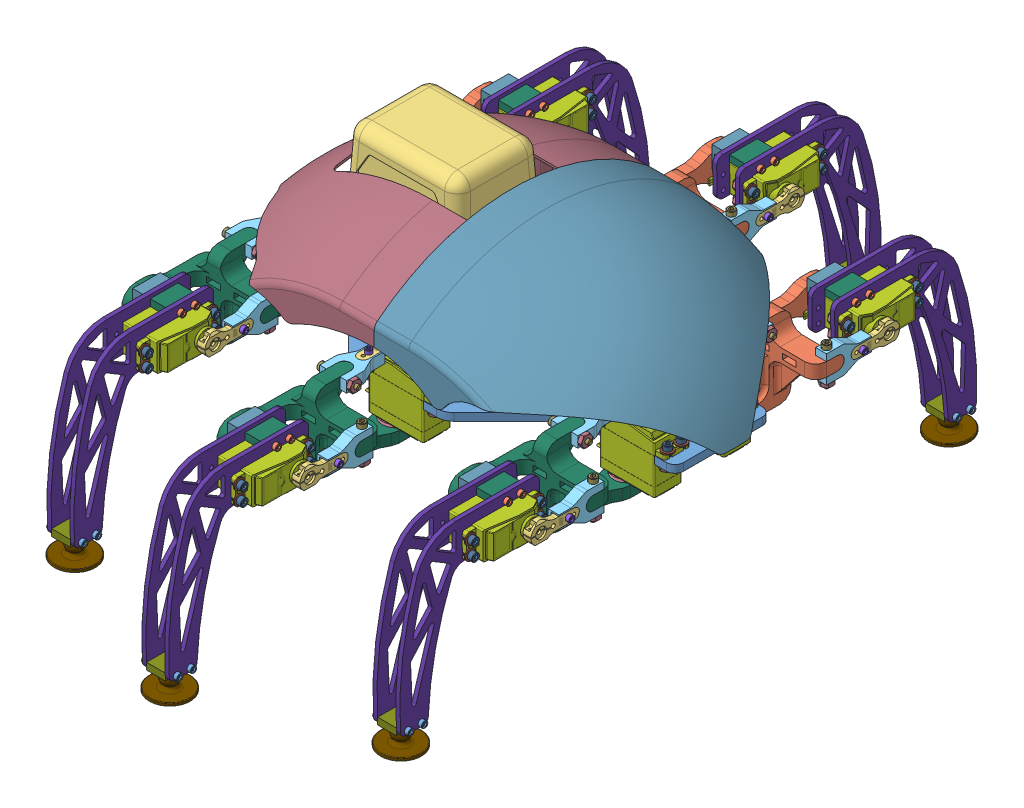
SolidWorks assembly Hexapod_(Small), configuration Défaut. Lengths in mm. (continued)
Mates (geometry in assembly coordinates):
- Coincident2: coincident anti-aligned: plane of Body_(Small)-5 through (-295 -5.601 0) normal (0 0 -1)
- Coincident3: coincident aligned: plane of Body_(Small)-5 through (-310 0 15.2) normal (0 1 0)
- Coincident4: coincident aligned: plane of Body_(Small)-5 through (0 0 50.6) normal (1 0 0)
- Coïncidente2: coincident anti-aligned: plane of arduinoMega-1 through (-199.11 -5.6 14.42) normal (0 1 0); plane of Body_(Small)-5 through (-310 -5.6 15.2) normal (0 -1 0)
- Coïncidente4: coincident anti-aligned: plane of Body_(Small)-5 through (-310 -5.6 15.2) normal (0 -1 0); plane of 12Channel PWM-1 through (-154.8 -5.6 -12.75) normal (0 1 0)
- Coïncidente5: coincident anti-aligned: plane of Body_(Small)-5 through (-310 -5.6 15.2) normal (0 -1 0); plane of DROK_090483.stp-1 through (-99 -5.6 15.2) normal (0 1 0)
- Parallèle4: parallel aligned: plane of Body_(Small)-5 through (0 0 50.6) normal (1 0 0); plane of 12Channel PWM-1 through (-132.7 -7.1 -12.75) normal (1 0 0)
- Concentric13: concentric aligned: cylinder of Body_(Small)-5 through (-154.8 0 43.15) axis (0 -1 0) radius 1.25; cylinder of 12Channel PWM-1 through (-154.8 -2.0645 43.15) axis (0 -1 0) radius 1.25
- Concentric17: concentric anti-aligned: circle of Body-1; circle of DROK_090483.stp-1
- Concentric18: concentric aligned: cylinder of Body_(Small)-5 through (-80.685 0 41.615) axis (0 -1 0) radius 1.45; cylinder of DROK_090483.stp-1 through (-80.685 -5.6 41.615) axis (0 -1 0) radius 1.585
- Concentric19: concentric aligned: cylinder of Body_(Small)-5 through (-175 0 -26.2) axis (0 -1 0) radius 1.6; circle of arduinoMega-1
- Concentric22: concentric aligned: cylinder of Body_(Small)-5 through (-223.22 0 49.91) axis (0 -1 0) radius 1.6; cylinder of arduinoMega-1 through (-223.22 -7.6 49.91) axis (0 -1 0) radius 1.6
- Concentric23: concentric anti-aligned: cylinder of Body_(Small)-5 through (-40.288 0 19.69) axis (0 -1 0) radius 1.45; cylinder of HX-SHCS 0.138-32x0.625x0.625-N-2 through (-40.288 35.2552 19.69) axis (0 1 0) radius 1.7526
- Concentric24: concentric anti-aligned: cylinder of Body_(Small)-5 through (-50.288 0 19.69) axis (0 -1 0) radius 1.45; cylinder of HX-SHCS 0.138-32x0.625x0.625-N-3 through (-50.288 35.2552 19.69) axis (0 1 0) radius 1.7526
- Coincident19: coincident anti-aligned: plane of Body_(Small)-5 through (-310 0 15.2) normal (0 1 0); plane of HX-SHCS 0.138-32x0.625x0.625-N-2 through (-40.288 0 16.8198) normal (0 -1 0)
- Coincident20: coincident anti-aligned: plane of Body_(Small)-5 through (-310 0 15.2) normal (0 1 0); plane of HX-SHCS 0.138-32x0.625x0.625-N-3 through (-47.8023 0 18.2549) normal (0 -1 0)
- Parallel10: parallel aligned: plane of Body_(Small)-5 through (0 0 50.6) normal (1 0 0); plane of HX-SHCS 0.138-32x0.625x0.625-N-3 through (-51.6723 1.8796 20.4892) normal (1 0 0)
- Parallel11: parallel aligned: plane of Body_(Small)-5 through (0 0 50.6) normal (1 0 0); plane of HX-SHCS 0.138-32x0.625x0.625-N-2 through (-41.6723 1.8796 18.8908) normal (1 0 0)
- Concentric25: concentric anti-aligned: cylinder of Body_(Small)-5 through (-50.288 0 10.71) axis (0 -1 0) radius 1.45; cylinder of HX-SHCS 0.138-32x0.625x0.625-N-4 through (-50.288 35.2552 10.71) axis (0 1 0) radius 1.7526
- Concentric26: concentric anti-aligned: cylinder of Body_(Small)-5 through (-40.288 0 10.71) axis (0 -1 0) radius 1.45; cylinder of HX-SHCS 0.138-32x0.625x0.625-N-5 through (-40.288 35.2552 10.71) axis (0 1 0) radius 1.7526
- Coincident23: coincident anti-aligned: plane of Body_(Small)-5 through (-310 0 15.2) normal (0 1 0); plane of HX-SHCS 0.138-32x0.625x0.625-N-5 through (-40.288 0 7.8398) normal (0 -1 0)
- Coincident24: coincident anti-aligned: plane of Body_(Small)-5 through (-310 0 15.2) normal (0 1 0); plane of HX-SHCS 0.138-32x0.625x0.625-N-4 through (-50.288 0 7.8398) normal (0 -1 0)
- Parallel12: parallel aligned: plane of Body_(Small)-5 through (0 0 50.6) normal (1 0 0); plane of HX-SHCS 0.138-32x0.625x0.625-N-5 through (-41.6723 1.8796 9.9108) normal (1 0 0)
- Parallel13: parallel aligned: plane of Body_(Small)-5 through (0 0 50.6) normal (1 0 0); plane of HX-SHCS 0.138-32x0.625x0.625-N-4 through (-51.6723 1.8796 9.9108) normal (1 0 0)
- Concentric27: concentric anti-aligned: cylinder of Body_(Small)-5 through (-170.288 0 -39.29) axis (0 -1 0) radius 1.45; cylinder of HX-SHCS 0.138-32x0.625x0.625-N-13 through (-214.94 40.2807 -39.09) axis (0 1 0) radius 1.7526
- Concentric29: concentric anti-aligned: cylinder of Body_(Small)-5 through (-160.288 0 69.69) axis (0 -1 0) radius 1.45; cylinder of HX-SHCS 0.138-32x0.625x0.625-N-7 through (-160.288 35.2552 69.69) axis (0 1 0) radius 1.7526
- Concentric30: concentric anti-aligned: cylinder of Body_(Small)-5 through (-170.288 0 69.69) axis (0 -1 0) radius 1.45; cylinder of HX-SHCS 0.138-32x0.625x0.625-N-6 through (-170.288 35.2552 69.69) axis (0 1 0) radius 1.7526
- Coincident27: coincident anti-aligned: plane of Body_(Small)-5 through (-310 0 15.2) normal (0 1 0); plane of HX-SHCS 0.138-32x0.625x0.625-N-7 through (-160.288 0 66.8198) normal (0 -1 0)
- Coincident28: coincident anti-aligned: plane of Body_(Small)-5 through (-310 0 15.2) normal (0 1 0); plane of HX-SHCS 0.138-32x0.625x0.625-N-6 through (-170.288 0 66.8198) normal (0 -1 0)
- Parallel14: parallel aligned: plane of Body_(Small)-5 through (0 0 50.6) normal (1 0 0); plane of HX-SHCS 0.138-32x0.625x0.625-N-6 through (-171.6723 1.8796 68.8908) normal (1 0 0)
- Parallel15: parallel aligned: plane of Body_(Small)-5 through (0 0 50.6) normal (1 0 0); plane of HX-SHCS 0.138-32x0.625x0.625-N-7 through (-161.6723 1.8796 68.8908) normal (1 0 0)
- Concentric31: concentric anti-aligned: cylinder of Body_(Small)-5 through (-170.288 0 -39.29) axis (0 -1 0) radius 1.45; cylinder of HX-SHCS 0.138-32x0.625x0.625-N-15 through (-170.288 35.2552 -39.29) axis (0 1 0) radius 1.7526
- Concentric32: concentric anti-aligned: cylinder of Body_(Small)-5 through (-160.288 0 -39.29) axis (0 -1 0) radius 1.45; cylinder of HX-SHCS 0.138-32x0.625x0.625-N-14 through (-160.288 35.2552 -39.29) axis (0 1 0) radius 1.7526
- Coincident31: coincident anti-aligned: plane of Body_(Small)-5 through (-310 0 15.2) normal (0 1 0); plane of HX-SHCS 0.138-32x0.625x0.625-N-15 through (-170.288 0 -42.1602) normal (0 -1 0)
- Coincident32: coincident anti-aligned: plane of Body_(Small)-5 through (-310 0 15.2) normal (0 1 0); plane of HX-SHCS 0.138-32x0.625x0.625-N-14 through (-160.288 0 -42.1602) normal (0 -1 0)
- Parallel16: parallel anti-aligned: plane of Body_(Small)-5 through (0 0 50.6) normal (1 0 0); plane of HX-SHCS 0.138-32x0.625x0.625-N-15 through (-168.9037 1.8796 -38.4908) normal (-1 0 0)
- Parallel17: parallel anti-aligned: plane of Body_(Small)-5 through (0 0 50.6) normal (1 0 0); plane of HX-SHCS 0.138-32x0.625x0.625-N-14 through (-158.9037 1.8796 -38.4908) normal (-1 0 0)
- Concentric33: concentric aligned: cylinder of Body_(Small)-5 through (-289.9 -5.601 19.3) axis (0 1 0) radius 1.45; cylinder of HX-SHCS 0.138-32x0.625x0.625-N-17 through (-289.9 35.2552 19.3) axis (0 1 0) radius 1.7526
- Concentric34: concentric aligned: circle of Body-1; cylinder of HX-SHCS 0.138-32x0.625x0.625-N-16 through (-279.9 35.2552 19.3) axis (0 1 0) radius 1.7526
- Concentric35: concentric aligned: cylinder of Body_(Small)-5 through (-289.9 -5.601 11.1) axis (0 1 0) radius 1.45; cylinder of HX-SHCS 0.138-32x0.625x0.625-N-18 through (-289.9 35.2552 11.1) axis (0 1 0) radius 1.7526
- Concentric36: concentric aligned: cylinder of Body_(Small)-5 through (-279.9 -5.601 11.1) axis (0 1 0) radius 1.45; cylinder of HX-SHCS 0.138-32x0.625x0.625-N-19 through (-279.9 35.2552 11.1) axis (0 1 0) radius 1.7526
- Coincident35: coincident anti-aligned: plane of Body_(Small)-5 through (-310 0 15.2) normal (0 1 0); plane of HX-SHCS 0.138-32x0.625x0.625-N-18 through (-289.9 0 8.2298) normal (0 -1 0)
- Coincident36: coincident anti-aligned: plane of Body_(Small)-5 through (-310 0 15.2) normal (0 1 0); plane of HX-SHCS 0.138-32x0.625x0.625-N-19 through (-279.9 0 8.2298) normal (0 -1 0)
- Coincident37: coincident anti-aligned: plane of Body_(Small)-5 through (-310 0 15.2) normal (0 1 0); plane of HX-SHCS 0.138-32x0.625x0.625-N-17 through (-287.4143 0 17.8649) normal (0 -1 0)
- Coincident38: coincident anti-aligned: plane of Body_(Small)-5 through (-310 0 15.2) normal (0 1 0); plane of HX-SHCS 0.138-32x0.625x0.625-N-16 through (-279.9 0 16.4298) normal (0 -1 0)
- Parallel18: parallel anti-aligned: plane of Body_(Small)-5 through (0 0 50.6) normal (1 0 0); plane of HX-SHCS 0.138-32x0.625x0.625-N-19 through (-278.5157 1.8796 11.8992) normal (-1 0 0)
- Parallel19: parallel anti-aligned: plane of Body_(Small)-5 through (0 0 50.6) normal (1 0 0); plane of HX-SHCS 0.138-32x0.625x0.625-N-18 through (-288.5157 1.8796 11.8992) normal (-1 0 0)
- Parallel20: parallel anti-aligned: plane of Body_(Small)-5 through (0 0 50.6) normal (1 0 0); plane of HX-SHCS 0.138-32x0.625x0.625-N-16 through (-278.5157 1.8796 20.0992) normal (-1 0 0)
- Parallel21: parallel anti-aligned: plane of Body_(Small)-5 through (0 0 50.6) normal (1 0 0); plane of HX-SHCS 0.138-32x0.625x0.625-N-17 through (-288.5157 1.8796 18.5008) normal (-1 0 0)
- Coincident40: coincident anti-aligned: plane of Body_(Small)-5 through (-310 -5.6 15.2) normal (0 -1 0); plane of MSHXNUT 0.138-32-D-N-60 through (-306.6748 -5.6 -15.08) normal (0 1 0)
- Coincident44: coincident anti-aligned: plane of Body_(Small)-5 through (-310 -5.6 15.2) normal (0 -1 0); plane of MSHXNUT 0.138-32-D-N-65 through (-306.6748 -5.6 -4.92) normal (0 1 0)
- Coincident47: coincident anti-aligned: plane of Body_(Small)-5 through (-310 -5.6 15.2) normal (0 -1 0); plane of MSHXNUT 0.138-32-D-N-75 through (-255.2144 -5.6 -21.9431) normal (0 1 0)
- Coincident48: coincident anti-aligned: plane of Body_(Small)-5 through (-310 -5.6 15.2) normal (0 -1 0); plane of MSHXNUT 0.138-32-D-N-70 through (-255.2144 -5.6 -11.7831) normal (0 1 0)
- Concentric41: concentric anti-aligned: cylinder of HX-SHCS 0.138-32x0.625x0.625-N-19 through (-279.9 35.2552 11.1) axis (0 1 0) radius 1.7526; circle of MSHXNUT 0.138-32-D-N-5
- Concentric42: concentric anti-aligned: cylinder of HX-SHCS 0.138-32x0.625x0.625-N-18 through (-289.9 35.2552 11.1) axis (0 1 0) radius 1.7526; circle of MSHXNUT 0.138-32-D-N-6
- Concentric43: concentric aligned: cylinder of arduinoMega-1 through (-175 -7.6 48.68) axis (0 -1 0) radius 1.6; cylinder of HX-SHCS 0.138-32x0.5x0.5-N-20 through (-175 -44.3552 48.68) axis (0 -1 0) radius 1.7526
- Concentric44: concentric aligned: cylinder of arduinoMega-1 through (-223.22 -7.6 49.91) axis (0 -1 0) radius 1.6; cylinder of HX-SHCS 0.138-32x0.5x0.5-N-23 through (-223.22 -44.3552 49.91) axis (0 -1 0) radius 1.7526
- Concentric45: concentric aligned: cylinder of arduinoMega-1 through (-223.22 -7.6 -32.56) axis (0 -1 0) radius 1.6; cylinder of HX-SHCS 0.138-32x0.5x0.5-N-21 through (-223.22 -44.3552 -32.56) axis (0 -1 0) radius 1.7526
- Concentric46: concentric aligned: cylinder of arduinoMega-1 through (-175 -7.6 -26.2) axis (0 -1 0) radius 1.6; cylinder of HX-SHCS 0.138-32x0.5x0.5-N-22 through (-175 -44.3552 -26.2) axis (0 -1 0) radius 1.7526
- Coincident58: coincident anti-aligned: plane of arduinoMega-1 through (-199.11 -9.1 14.42) normal (0 -1 0); plane of HX-SHCS 0.138-32x0.5x0.5-N-20 through (-172.5143 -9.1 47.2449) normal (0 1 0)
- Coincident59: coincident anti-aligned: plane of arduinoMega-1 through (-199.11 -9.1 14.42) normal (0 -1 0); plane of HX-SHCS 0.138-32x0.5x0.5-N-22 through (-172.5143 -9.1 -27.6351) normal (0 1 0)
- Coincident60: coincident anti-aligned: plane of arduinoMega-1 through (-199.11 -9.1 14.42) normal (0 -1 0); plane of HX-SHCS 0.138-32x0.5x0.5-N-23 through (-223.22 -9.1 47.0398) normal (0 1 0)
- Coincident61: coincident anti-aligned: plane of arduinoMega-1 through (-199.11 -9.1 14.42) normal (0 -1 0); plane of HX-SHCS 0.138-32x0.5x0.5-N-21 through (-223.22 -9.1 -29.6898) normal (0 1 0)
- Concentric47: concentric anti-aligned: cylinder of HX-SHCS 0.138-32x0.5x0.5-N-21 through (-223.22 -44.3552 -32.56) axis (0 -1 0) radius 1.7526; circle of MSHXNUT 0.112-40-S-N-2
- Concentric48: concentric anti-aligned: cylinder of HX-SHCS 0.138-32x0.5x0.5-N-23 through (-223.22 -44.3552 49.91) axis (0 -1 0) radius 1.7526; circle of MSHXNUT 0.112-40-S-N-3
- Concentric49: concentric anti-aligned: cylinder of HX-SHCS 0.138-32x0.5x0.5-N-22 through (-175 -44.3552 -26.2) axis (0 -1 0) radius 1.7526; circle of MSHXNUT 0.112-40-S-N-4
- Concentric50: concentric anti-aligned: cylinder of HX-SHCS 0.138-32x0.5x0.5-N-20 through (-175 -44.3552 48.68) axis (0 -1 0) radius 1.7526; circle of MSHXNUT 0.112-40-S-N-5
- Coincident62: coincident anti-aligned: plane of Body_(Small)-5 through (-310 0 15.2) normal (0 1 0); plane of MSHXNUT 0.112-40-D-N-109 through (-181.35 0 48.68) normal (0 -1 0)
- Coincident63: coincident anti-aligned: plane of Body_(Small)-5 through (-310 0 15.2) normal (0 1 0); plane of MSHXNUT 0.112-40-D-N-108 through (-181.35 0 -26.2) normal (0 -1 0)
- Coincident64: coincident anti-aligned: plane of Body_(Small)-5 through (-310 0 15.2) normal (0 1 0); plane of MSHXNUT 0.112-40-D-N-107 through (-229.57 0 49.91) normal (0 -1 0)
- Coincident65: coincident anti-aligned: plane of Body_(Small)-5 through (-310 0 15.2) normal (0 1 0); plane of MSHXNUT 0.112-40-D-N-106 through (-229.57 0 -32.56) normal (0 -1 0)
- Parallel28: parallel anti-aligned: plane of Body_(Small)-5 through (-310 0 15.2) normal (-1 0 0); plane of MSHXNUT 0.112-40-D-N-107 through (-220.045 0 48.0769) normal (1 0 0)
- Parallel30: parallel aligned: plane of Body_(Small)-5 through (-310 0 15.2) normal (-1 0 0); plane of MSHXNUT 0.112-40-D-N-106 through (-226.395 0 -34.3931) normal (-1 0 0)
- Parallel31: parallel aligned: plane of Body_(Small)-5 through (-310 0 15.2) normal (-1 0 0); plane of MSHXNUT 0.112-40-D-N-108 through (-178.175 0 -28.0331) normal (-1 0 0)
- Parallel32: parallel aligned: plane of Body_(Small)-5 through (-310 0 15.2) normal (-1 0 0); plane of MSHXNUT 0.112-40-D-N-109 through (-178.175 0 46.8469) normal (-1 0 0)
- Parallel33: parallel aligned: plane of arduinoMega-1 through (-225.76 -9.1 63.91) normal (-1 0 0); plane of HX-SHCS 0.138-32x0.5x0.5-N-23 through (-221.8357 -10.9796 49.1108) normal (-1 0 0)
- Parallel34: parallel aligned: plane of arduinoMega-1 through (-225.76 -9.1 63.91) normal (-1 0 0); plane of HX-SHCS 0.138-32x0.5x0.5-N-20 through (-173.6157 -10.9796 47.8808) normal (-1 0 0)
- Parallel35: parallel aligned: plane of arduinoMega-1 through (-225.76 -9.1 63.91) normal (-1 0 0); plane of HX-SHCS 0.138-32x0.5x0.5-N-22 through (-173.6157 -10.9796 -26.9992) normal (-1 0 0)
- Parallel36: parallel aligned: plane of arduinoMega-1 through (-225.76 -9.1 63.91) normal (-1 0 0); plane of HX-SHCS 0.138-32x0.5x0.5-N-21 through (-221.8357 -10.9796 -33.3592) normal (-1 0 0)
- Concentric51: concentric aligned: cylinder of DROK_090483.stp-1 through (-117.315 -5.6 -11.215) axis (0 -1 0) radius 1.585; cylinder of HX-SHCS 0.138-32x0.5x0.5-N-24 through (-117.315 -42.0552 -11.215) axis (0 -1 0) radius 1.7526
- Coincident74: coincident anti-aligned: plane of DROK_090483.stp-1 through (-99 -6.8 15.2) normal (0 -1 0); plane of HX-SHCS 0.138-32x0.5x0.5-N-24 through (-114.8293 -6.8 -12.6501) normal (0 1 0)
- Parallel37: parallel aligned: plane of DROK_090483.stp-1 through (-120.5 -5.6 45.2) normal (-1 0 0); plane of HX-SHCS 0.138-32x0.5x0.5-N-24 through (-115.9307 -8.6796 -12.0142) normal (-1 0 0)
- Concentric52: concentric anti-aligned: cylinder of HX-SHCS 0.138-32x0.5x0.5-N-24 through (-117.315 -42.0552 -11.215) axis (0 -1 0) radius 1.7526; circle of MSHXNUT 0.112-40-S-N-6
- Coincident76: coincident anti-aligned: plane of Body_(Small)-5 through (-310 0 15.2) normal (0 1 0); plane of MSHXNUT 0.112-40-D-N-110 through (-123.665 0 -11.215) normal (0 -1 0)
- Parallel38: parallel anti-aligned: plane of Body_(Small)-5 through (0 0 50.6) normal (1 0 0); plane of MSHXNUT 0.112-40-D-N-110 through (-120.49 0 -13.0481) normal (-1 0 0)
- Concentric53: concentric anti-aligned: cylinder of Body_(Small)-5 through (-70 -5.6 -9.3) axis (0 1 0) radius 1.375; cylinder of 1_4_Round_Aluminum_Standoff.step-1 through (-70 6.35 -9.3) axis (0 -1 0) radius 3.1712
- Coincident78: coincident anti-aligned: plane of Body_(Small)-5 through (-310 0 15.2) normal (0 1 0); plane of 1_4_Round_Aluminum_Standoff.step-1 through (-70 0 -9.3) normal (0 -1 0)
- Coincident83: coincident anti-aligned: plane of Body_(Small)-5 through (-310 -5.6 15.2) normal (0 -1 0); plane of MSHXNUT 0.112-40-D-N-117 through (-76.35 -5.6 -9.3) normal (0 1 0)
- Parallel40: parallel aligned: plane of Body_(Small)-5 through (0 0 50.6) normal (1 0 0); plane of MSHXNUT 0.112-40-D-N-117 through (-66.825 -5.6 -7.4669) normal (1 0 0)
- Concentric56: concentric aligned: cylinder of 12Channel PWM-1 through (-154.8 -2.0645 -12.75) axis (0 -1 0) radius 1.25; cylinder of HX-SHCS 0.112-40x0.5x0.5-N-32 through (-154.8 -41.6948 -12.75) axis (0 -1 0) radius 1.4224
- Coincident85: coincident anti-aligned: plane of 12Channel PWM-1 through (-154.8 -7.1 -12.75) normal (0 -1 0); plane of HX-SHCS 0.112-40x0.5x0.5-N-32 through (-154.8 -7.1 -15.0741) normal (0 1 0)
- Parallel41: parallel aligned: plane of 12Channel PWM-1 through (-132.7 -7.1 -12.75) normal (1 0 0); plane of HX-SHCS 0.112-40x0.5x0.5-N-32 through (-155.9938 -8.6494 -12.0608) normal (1 0 0)
- Concentric57: concentric anti-aligned: cylinder of HX-SHCS 0.112-40x0.5x0.5-N-32 through (-154.8 -41.6948 -12.75) axis (0 -1 0) radius 1.4224; circle of MSHXNUT 0.112-40-D-N-68
- Coincident88: coincident anti-aligned: plane of Body_(Small)-5 through (-310 0 15.2) normal (0 1 0); plane of MSHXNUT 0.112-40-D-N-124 through (-161.15 0 -12.75) normal (0 -1 0)
- Parallel42: parallel aligned: plane of Body_(Small)-5 through (0 0 50.6) normal (1 0 0); plane of MSHXNUT 0.112-40-D-N-124 through (-151.625 0 -14.5831) normal (1 0 0)
- Parallel43: parallel aligned: plane of raspberryPi3B-1 through (-66.5 7.65 43.2) normal (1 0 0); plane of Body_(Small)-5 through (0 0 50.6) normal (1 0 0)
- Concentric64: concentric aligned: circle of raspberryPi3B-1; cylinder of HX-SHCS 0.112-40x1x0.75-N-47 through (-70 42.2448 -9.3) axis (0 1 0) radius 1.4224
- Coincident92: coincident aligned: cylinder of HX-SHCS 0.112-40x1x0.75-N-47 through (-70 42.2448 -9.3) axis (0 1 0) radius 1.4224; circle of machine screw nut hex_ai-114
- Concentric65: concentric anti-aligned: cylinder of 1_4_Round_Aluminum_Standoff.step-3 through (-70 6.35 39.7) axis (0 -1 0) radius 3.1712; cylinder of HX-SHCS 0.112-40x1x0.75-N-52 through (-70 42.2448 39.7) axis (0 1 0) radius 1.4224
- Coincident93: coincident anti-aligned: plane of raspberryPi3B-1 through (-109 6.35 15.2) normal (0 -1 0); plane of 1_4_Round_Aluminum_Standoff.step-1 through (-70 6.35 -9.3) normal (0 1 0)
- Coincident96: coincident anti-aligned: plane of raspberryPi3B-1 through (-109 7.65 15.2) normal (0 1 0); plane of HX-SHCS 0.112-40x1x0.75-N-47 through (-68.2097 7.65 -10.7819) normal (0 -1 0)
- Coincident97: coincident anti-aligned: plane of Body_(Small)-5 through (-310 0 15.2) normal (0 1 0); plane of 1_4_Round_Aluminum_Standoff.step-5 through (-182.4233 0 -9.675) normal (0 -1 0)
- Concentric68: concentric anti-aligned: cylinder of HX-SHCS 0.112-40x1x0.75-N-61 through (-182.4233 -40.1948 -9.675) axis (0 -1 0) radius 1.4224; cylinder of Body_(Small)-5 through (-182.4233 -5.6 -9.675) axis (0 1 0) radius 1.45
- Coincident109: coincident anti-aligned: plane of Body_(Small)-5 through (-310 0 15.2) normal (0 1 0); plane of Shell_(Front)-4 through (-339.15 0 173.95) normal (0 -1 0)
- Concentric71: concentric aligned: circle of Body_V2-5; circle of Shell_front-2
- Concentric72: concentric anti-aligned: circle of Body_V2-5; circle of Shell_front-2
- Coincident112: coincident anti-aligned: plane of Body_(Small)-5 through (-310 0 15.2) normal (0 1 0); plane of Shell_(Back)-3 through (29.15 0 -143.55) normal (0 -1 0)
- Concentric74: concentric anti-aligned: circle of Body_V2-5; circle of Shell_back-3
- Coincident113: coincident anti-aligned: plane of Body_(Small)-5 through (-55 -5.6 -0.2) normal (0 0 -1); plane of Foot+Femur_(Mirror)-6/DS3225MG-3 through (-54.2 -65.0799 -0.2) normal (0 0 1)
- Coincident114: coincident anti-aligned: plane of Body_(Small)-5 through (-15 -5.6 -0.2) normal (-1 0 0); plane of Foot+Femur_(Mirror)-6/DS3225MG-3 through (-15 -65.0799 -1.2) normal (1 0 0)
- Coincident115: coincident anti-aligned: plane of Body_(Small)-5 through (-310 0 15.2) normal (0 1 0); plane of Foot+Femur_(Mirror)-6/DS3225MG-3 through (-54.2 0 -1.2) normal (0 -1 0)
- Coincident116: coincident anti-aligned: plane of Body_(Small)-5 through (-135 -5.6 -50.2) normal (-1 0 0); plane of Foot+Femur_(Mirror)-7/DS3225MG-3 through (-135 -65.0799 -51.2) normal (1 0 0)
- Coincident117: coincident anti-aligned: plane of Body_(Small)-5 through (-310 0 15.2) normal (0 1 0); plane of Foot+Femur_(Mirror)-7/DS3225MG-3 through (-174.2 0 -51.2) normal (0 -1 0)
- Coincident118: coincident anti-aligned: plane of Body_(Small)-5 through (-175 -5.6 -50.2) normal (0 0 -1); plane of Foot+Femur_(Mirror)-7/DS3225MG-3 through (-174.2 -65.0799 -50.2) normal (0 0 1)
- Coincident119: coincident anti-aligned: plane of Body_(Small)-5 through (-254.8 -5.601 0) normal (-1 0 0); plane of Foot+Femur_(Mirror)-8/DS3225MG-3 through (-254.8 -65.0799 -1) normal (1 0 0)
- Coincident120: coincident anti-aligned: plane of Body_(Small)-5 through (-310 0 15.2) normal (0 1 0); plane of Foot+Femur_(Mirror)-8/DS3225MG-3 through (-294 0 -1) normal (0 -1 0)
- Coincident121: coincident anti-aligned: plane of Body_(Small)-5 through (-295 -5.601 0) normal (0 0 -1); plane of Foot+Femur_(Mirror)-8/DS3225MG-3 through (-294 -65.0799 0) normal (0 0 1)
- Coincident122: coincident anti-aligned: plane of Body_(Small)-5 through (-254.8 -5.601 30.4) normal (-1 0 0); plane of Foot+Femur-1/DS3225MG-3 through (-254.8 -65.0799 49.8) normal (1 0 0)
- Coincident123: coincident anti-aligned: plane of Body_(Small)-5 through (-310 0 15.2) normal (0 1 0); plane of Foot+Femur-1/DS3225MG-3 through (-294 0 49.8) normal (0 -1 0)
- Coincident124: coincident anti-aligned: plane of Body_(Small)-5 through (-295 -5.601 30.4) normal (0 0 1); plane of Foot+Femur-1/DS3225MG-3 through (-255.8 -65.0799 30.4) normal (0 0 -1)
- Coincident125: coincident anti-aligned: plane of Body_(Small)-5 through (-175 -5.6 80.6) normal (0 0 1); plane of Foot+Femur-3/DS3225MG-3 through (-135.8 -65.0799 80.6) normal (0 0 -1)
- Coincident126: coincident anti-aligned: plane of Body_(Small)-5 through (-310 0 15.2) normal (0 1 0); plane of Foot+Femur-3/DS3225MG-3 through (-174 0 100) normal (0 -1 0)
- Coincident127: coincident anti-aligned: plane of Body_(Small)-5 through (-175 -5.6 80.6) normal (1 0 0); plane of Foot+Femur-3/DS3225MG-3 through (-175 -65.0799 81.6) normal (-1 0 0)
- Coincident128: coincident anti-aligned: plane of Body_(Small)-5 through (-310 0 15.2) normal (0 1 0); plane of Foot+Femur-4/DS3225MG-3 through (-54 0 50) normal (0 -1 0)
- Coincident129: coincident anti-aligned: plane of Body_(Small)-5 through (-55 -5.6 30.6) normal (0 0 1); plane of Foot+Femur-4/DS3225MG-3 through (-15.8 -65.0799 30.6) normal (0 0 -1)
- Coincident130: coincident anti-aligned: plane of Body_(Small)-5 through (-55 -5.6 30.6) normal (1 0 0); plane of Foot+Femur-4/DS3225MG-3 through (-55 -65.0799 31.6) normal (-1 0 0)
- Distance1: distance = 15 mm anti-aligned: plane of Battery_holder-1 through (-237.0983 97.5528 -15) normal (0 0 -1)
- Parallel44: parallel aligned: plane of Body_(Small)-5 through (-310 0 -20.2) normal (0 0 -1); plane of Battery_holder-1 through (-237.0983 97.5528 -15) normal (0 0 -1)
- Coincident133: coincident anti-aligned: plane of 1_4_Round_Aluminum_Standoff.step-7 through (-231.7733 6.35 -9.675) normal (0 1 0); plane of Battery_holder-1 through (-192.0983 6.35 30) normal (0 -1 0)
- Coincident134: coincident anti-aligned: plane of Body_(Small)-5 through (-310 -5.6 15.2) normal (0 -1 0); plane of HX-SHCS 0.112-40x1x0.75-N-61 through (-182.1683 -5.6 -7.3649) normal (0 1 0)
- Concentric77: concentric aligned: cylinder of 1_4_Round_Aluminum_Standoff.step-5 through (-182.4233 6.35 -9.675) axis (0 -1 0) radius 3.1712; cylinder of HX-SHCS 0.112-40x1x0.75-N-61 through (-182.4233 -40.1948 -9.675) axis (0 -1 0) radius 1.4224
- Concentric78: concentric aligned: cylinder of HX-SHCS 0.112-40x1x0.75-N-61 through (-182.4233 -40.1948 -9.675) axis (0 -1 0) radius 1.4224; cylinder of MSHXNUT 0.112-40-D-N-131 through (-182.4233 15.1892 -9.675) axis (0 -1 0) radius 1.1303
- Coincident135: coincident anti-aligned: plane of Battery_holder-1 through (-192.0983 12.7 26) normal (0 1 0); plane of MSHXNUT 0.112-40-D-N-131 through (-177.1073 12.7 -6.2019) normal (0 -1 0)
- Concentric80: concentric aligned: cylinder of Body_(Small)-5 through (-96.4645 -5.6 -32.1223) axis (0 1 0) radius 1.45; cylinder of Shell_(Back)-3 through (-96.4645 0 -32.1223) axis (0 1 0) radius 1.45
